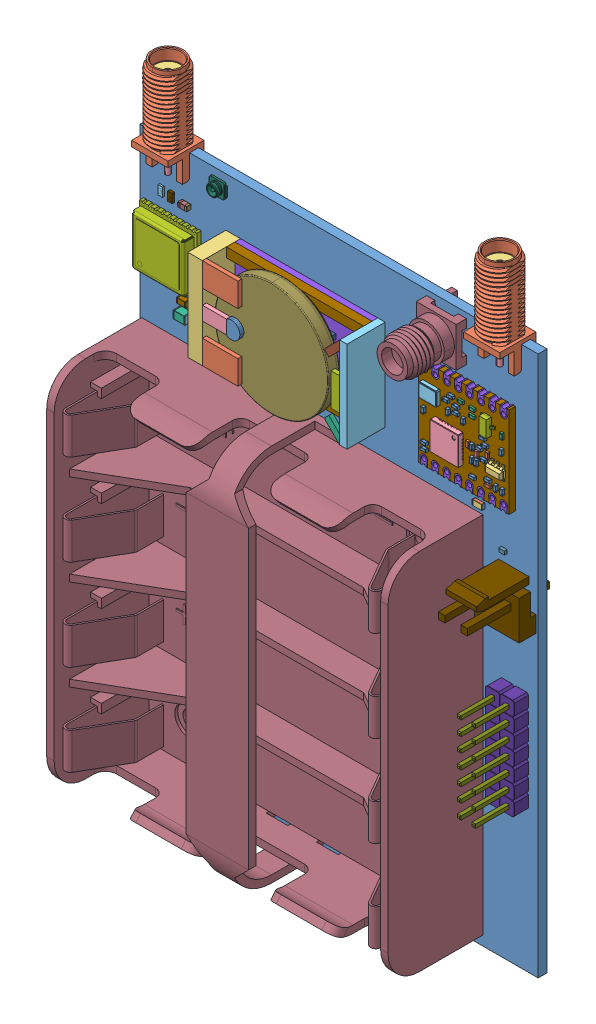
SolidWorks assembly Печатная плата Peggy Tracker степ, configuration По умолчанию. Lengths in mm.
Overall size (70 108.1 20.64).
358 component instances, 81 part files, 0 mates.
Components (placement in the parent):
- Печатная плата Peggy Tracker.step-1: Печатная плата Peggy Tracker.step [Default] at origin size (70 108.1 20.64)
  - Board.step-1: Board.step [Default] at origin size (70 95 1.56)
    - Open CASCADE STEP translator 6.8 1.1.1.step-1: Open CASCADE STEP translator 6.8 1.1.1.step [Default] at (0 0 -1.5596) size (70 95 1.56)
  - XW4.step-1: XW4.step [Default] at origin size (6.87 17.48 6.87)
    - SMA_female_edge_6.5x6.5.step-1: SMA_female_edge_6.5x6.5.step [Default] at (63.8984 92.1251 0.2) x (-1 0 0) z (0 0 1) size (6.87 17.48 6.87)
      - SMA_female_edge_6.5x6.5(2)^SMA_female_edge_6.5x6.5.step-1: SMA_female_edge_6.5x6.5(2)^SMA_female_edge_6.5x6.5.step [Default] at origin size (6.87 17.48 6.87)
        - Body^SMA_female_edge_6.5x6.5(2)_SMA_female_edge_6.5x6.5.step-1: Body^SMA_female_edge_6.5x6.5(2)_SMA_female_edge_6.5x6.5.step [Default] at (0 -4 0.45) x (0 0 1) z (0 -1 0) size (6.87 6.87 17.29)
        - Dielectric^SMA_female_edge_6.5x6.5(2)_SMA_female_edge_6.5x6.5.step-1: Dielectric^SMA_female_edge_6.5x6.5(2)_SMA_female_edge_6.5x6.5.step [Default] at (0 -4 0.45) x (0 0 1) z (0 -1 0) size (4.25 4.25 11.54)
        - Pin^SMA_female_edge_6.5x6.5(2)_SMA_female_edge_6.5x6.5.step-1: Pin^SMA_female_edge_6.5x6.5(2)_SMA_female_edge_6.5x6.5.step [Default] at (0 -4 0.45) x (0 0 1) z (0 -1 0) size (1.27 1.27 15.54)
  - C21.step-1: C21.step [Default] at origin size (1.6 0.8 0.3)
    - SW3dPS-0603_SMD_Capacitor.step-1: SW3dPS-0603_SMD_Capacitor.step [Default] at (25.6001 31.0999 -1.5596) x (1 0 0) z (0 1 0) size (1.6 0.3 0.8)
  - C20.step-1: C20.step [Default] at origin size (3.2 1.6 1)
    - SW3dPS-1206_SMD_Capacitor.step-1: SW3dPS-1206_SMD_Capacitor.step [Default] at (30.5 25 -1.5596) x (1 0 0) z (0 1 0) size (3.2 1 1.6)
  - C19.step-1: C19.step [Default] at origin size (1.6 0.8 0.3)
    - SW3dPS-0603_SMD_Capacitor.step-1: SW3dPS-0603_SMD_Capacitor.step [Default] at (27.9999 46.9001 -1.5596) x (-1 0 0) z (0 -1 0) size (1.6 0.3 0.8)
  - C18.step-1: C18.step [Default] at origin size (0.8 1.6 0.3)
    - SW3dPS-0603_SMD_Capacitor.step-1: SW3dPS-0603_SMD_Capacitor.step [Default] at (40.0999 43.0999 -1.5596) x (0 -1 0) z (1 0 0) size (1.6 0.3 0.8)
  - C17.step-1: C17.step [Default] at origin size (0.8 1.6 0.3)
    - SW3dPS-0603_SMD_Capacitor.step-1: SW3dPS-0603_SMD_Capacitor.step [Default] at (39.9001 34.9001 -1.5596) x (0 1 0) z (-1 0 0) size (1.6 0.3 0.8)
  - C16.step-1: C16.step [Default] at origin size (1.6 0.8 0.3)
    - SW3dPS-0603_SMD_Capacitor.step-1: SW3dPS-0603_SMD_Capacitor.step [Default] at (22.1999 32.8001 -1.5596) x (-1 0 0) z (0 -1 0) size (1.6 0.3 0.8)
  - DD1.step-1: DD1.step [Default] at origin size (10.1 9.7 2.7)
    - MAX-M8C-0.step-1: MAX-M8C-0.step [Default] at (5.7001 79.2999 0) x (0 1 0) z (1 0 0) size (9.7 2.7 10.1)
  - ZQ2.step-1: ZQ2.step [Default] at origin size (3.22 1.52 0.91)
    - User_Library-ABS07.step-1: User_Library-ABS07.step [Default] at (18.5999 54.9001 -1.5596) x (-1 0 0) z (0 -1 0) size (3.22 0.91 1.52)
      - User_Library-ABS07_ABS07_Body_2.step-1: User_Library-ABS07_ABS07_Body_2.step [Default] x (1 0 0) z (0 1 0) size (3.2 1.5 0.85)
      - User_Library-ABS07_ABS07_Body2_2.step-1: User_Library-ABS07_ABS07_Body2_2.step [Default] x (-1 0 0) z (0 1 0) size (3 1.3 0.05)
      - User_Library-ABS07_ABS07_Beschriftung_2.step-1: User_Library-ABS07_ABS07_Beschriftung_2.step [Default] x (-1 0 0) z (0 1 0) size (2.05 0.49 0.06)
      - User_Library-ABS07_ABS07_Pads_2.step-1: User_Library-ABS07_ABS07_Pads_2.step [Default] x (1 0 0) z (0 1 0) size (3.22 1.52 0.25)
  - ZQ1.step-1: ZQ1.step [Default] at origin size (3.18 5 1.11)
    - ABM3B.step-1: ABM3B.step [Default] at (21.4001 38.8001 -1.5596) x (0 -1 0) z (1 0 0) size (5 1.11 3.17)
  - XW3.step-1: XW3.step [Default] at origin size (7.01 7.53 13.48)
    - SMA_connector.step-1: SMA_connector.step [Default] at (53.9001 90.6 0) size (7.01 7.53 13.48)
      - User_Library-SMA_Stehend_Amp_132134RP-1_1.step-1: User_Library-SMA_Stehend_Amp_132134RP-1_1.step [Default] at origin size (7.01 7.53 13.48)
      - User_Library-SMA_Stehend_Amp_132134RP-1_2.step-1: User_Library-SMA_Stehend_Amp_132134RP-1_2.step [Default] at origin size (1.27 1.27 4.71)
  - XW2.step-1: XW2.step [Default] at origin size (3.01 2.86 1.29)
    - IPX.step-1: IPX.step [Default] at (13.8501 92.4001 1.27) size (3.01 2.86 1.29)
  - XW1.step-1: XW1.step [Default] at origin size (6.87 17.48 6.87)
    - SMA_female_edge_6.5x6.5.step-1: SMA_female_edge_6.5x6.5.step [Default] at (5.5484 92.1251 0.2) x (-1 0 0) z (0 0 1) size (6.87 17.48 6.87)
      - SMA_female_edge_6.5x6.5(2)^SMA_female_edge_6.5x6.5.step-1: SMA_female_edge_6.5x6.5(2)^SMA_female_edge_6.5x6.5.step [Default] at origin size (6.87 17.48 6.87)
        - Body^SMA_female_edge_6.5x6.5(2)_SMA_female_edge_6.5x6.5.step-1: Body^SMA_female_edge_6.5x6.5(2)_SMA_female_edge_6.5x6.5.step [Default] at (0 -4 0.45) x (0 0 1) z (0 -1 0) size (6.87 6.87 17.29)
        - Dielectric^SMA_female_edge_6.5x6.5(2)_SMA_female_edge_6.5x6.5.step-1: Dielectric^SMA_female_edge_6.5x6.5(2)_SMA_female_edge_6.5x6.5.step [Default] at (0 -4 0.45) x (0 0 1) z (0 -1 0) size (4.25 4.25 11.54)
        - Pin^SMA_female_edge_6.5x6.5(2)_SMA_female_edge_6.5x6.5.step-1: Pin^SMA_female_edge_6.5x6.5(2)_SMA_female_edge_6.5x6.5.step [Default] at (0 -4 0.45) x (0 0 1) z (0 -1 0) size (1.27 1.27 15.54)
  - X5.step-1: X5.step [Default] at origin size (5.08 17.78 11.54)
    - PLD-14.step-1: PLD-14.step [Default] at (64.5301 25.9799 0) x (0 -1 0) z (0 0 1) size (17.78 5.08 11.54)
      - ____________.step-1: ____________.step [Default] at (-12.7 0 -3) size (0.64 0.64 11.54)
      - _________.step-1: _________.step [Default] at (-5.1324 2.5342 -0.0112) size (2.54 2.54 2.54)
      - ____________.step-2: ____________.step [Default] at (-7.62 2.54 -3) size (0.64 0.64 11.54)
      - _________.step-2: _________.step [Default] at (-12.7524 -0.0058 -0.0112) size (2.54 2.54 2.54)
      - ____________.step-3: ____________.step [Default] at (-15.24 2.54 -3) size (0.64 0.64 11.54)
      - _________.step-3: _________.step [Default] at (-10.2124 2.5342 -0.0112) size (2.54 2.54 2.54)
      - ____________.step-4: ____________.step [Default] at (-12.7 2.54 -3) size (0.64 0.64 11.54)
      - ____________.step-5: ____________.step [Default] at (-10.16 2.54 -3) size (0.64 0.64 11.54)
      - ____________.step-6: ____________.step [Default] at (-15.24 0 -3) size (0.64 0.64 11.54)
      - ____________.step-7: ____________.step [Default] at (0 2.54 -3) size (0.64 0.64 11.54)
      - ____________.step-8: ____________.step [Default] at (-7.62 0 -3) size (0.64 0.64 11.54)
      - _________.step-4: _________.step [Default] at (-5.1324 -0.0058 -0.0112) size (2.54 2.54 2.54)
      - _________.step-5: _________.step [Default] at (-2.5924 -0.0058 -0.0112) size (2.54 2.54 2.54)
      - ____________.step-9: ____________.step [Default] at (-2.54 0 -3) size (0.64 0.64 11.54)
      - ____________.step-10: ____________.step [Default] at (-5.08 0 -3) size (0.64 0.64 11.54)
      - _________.step-6: _________.step [Default] at (-0.0524 2.5342 -0.0112) size (2.54 2.54 2.54)
      - _________.step-7: _________.step [Default] at (-7.6724 2.5342 -0.0112) size (2.54 2.54 2.54)
      - ____________.step-11: ____________.step [Default] at (-5.08 2.54 -3) size (0.64 0.64 11.54)
      - _________.step-8: _________.step [Default] at (-7.6724 -0.0058 -0.0112) size (2.54 2.54 2.54)
      - _________.step-9: _________.step [Default] at (-15.2924 2.5342 -0.0112) size (2.54 2.54 2.54)
      - ____________.step-12: ____________.step [Default] at (-2.54 2.54 -3) size (0.64 0.64 11.54)
      - ____________.step-13: ____________.step [Default] at (0 0 -3) size (0.64 0.64 11.54)
      - _________.step-10: _________.step [Default] at (-10.2124 -0.0058 -0.0112) size (2.54 2.54 2.54)
      - _________.step-11: _________.step [Default] at (-15.2924 -0.0058 -0.0112) size (2.54 2.54 2.54)
      - _________.step-12: _________.step [Default] at (-2.5924 2.5342 -0.0112) size (2.54 2.54 2.54)
      - _________.step-13: _________.step [Default] at (-12.7524 2.5342 -0.0112) size (2.54 2.54 2.54)
      - _________.step-14: _________.step [Default] at (-0.0524 -0.0058 -0.0112) size (2.54 2.54 2.54)
      - ____________.step-14: ____________.step [Default] at (-10.16 0 -3) size (0.64 0.64 11.54)
  - X4.step-1: X4.step [Default] at origin size (7.86 8.5 14.4)
    - 1-1123723-2.step-1: 1-1123723-2.step [Default] at (65.7 57.0999 3) x (1 0 0) z (0 0 1) size (7.86 8.5 14.4)
  - X2.step-1: X2.step [Default] at origin size (28 20 6.7)
    - 6036059248.step-1: 6036059248.step [Default] at (22.75 78.4 6) size (3 3 0.7)
      - Extruded.step-1: Extruded.step [Default] at origin size (3 3 0.7)
    - 6036054288.step-1: 6036054288.step [Default] at (20.7815 72.4945 6) size (6.22 4.19 0.7)
      - Extruded-0.step-1: Extruded-0.step [Default] at origin size (6.22 4.19 0.7)
    - 6036054288.step-2: 6036054288.step [Default] at (20.7815 84.3045 6) size (6.22 4.19 0.7)
      - Extruded-0.step-1: Extruded-0.step [Default] at origin size (6.22 4.19 0.7)
    - 6036054608.step-1: 6036054608.step [Default] at (16.385 78.3995 0) size (2.57 16 6.7)
      - Extruded-1.step-1: Extruded-1.step [Default] at origin size (2.57 16 6.7)
    - 6036055008.step-1: 6036055008.step [Default] at (19.7818 78.4135 6) size (4.22 2.41 0.7)
      - Extruded-2.step-1: Extruded-2.step [Default] at origin size (4.22 2.41 0.7)
    - 6036055248.step-1: 6036055248.step [Default] at (42.4492 78.3995 0) size (1.3 16 6.7)
      - Extruded-3.step-1: Extruded-3.step [Default] at origin size (1.3 16 6.7)
    - 6036055568.step-1: 6036055568.step [Default] at (40.5305 72.1757 6) size (2.54 3.55 0.7)
      - Extruded-4.step-1: Extruded-4.step [Default] at origin size (2.54 3.55 0.7)
    - 6036055968.step-1: 6036055968.step [Default] at (41.0382 78.0825 6) size (1.52 5.71 0.7)
      - Extruded-5.step-1: Extruded-5.step [Default] at origin size (1.52 5.71 0.7)
    - 6036056288.step-1: 6036056288.step [Default] at (29.7354 78.3995 0) size (24.13 16 1)
      - Extruded-6.step-1: Extruded-6.step [Default] at origin size (24.13 16 1)
    - 6036056848.step-1: 6036056848.step [Default] at (29.735 85.575 0) size (24.13 1.65 2.5)
      - Extruded-7.step-1: Extruded-7.step [Default] at origin size (24.13 1.65 2.5)
    - 6036056848.step-2: 6036056848.step [Default] at (29.7356 71.2237 0) size (24.13 1.65 2.5)
      - Extruded-7.step-1: Extruded-7.step [Default] at origin size (24.13 1.65 2.5)
    - 6036057568.step-1: 6036057568.step [Default] at (30.6875 75.4163 0) size (9.53 0.89 2.5)
      - Extruded-8.step-1: Extruded-8.step [Default] at origin size (9.53 0.89 2.5)
    - 6036057568.step-2: 6036057568.step [Default] at (30.6875 80.8773 0) size (9.53 0.89 2.5)
      - Extruded-8.step-1: Extruded-8.step [Default] at origin size (9.53 0.89 2.5)
    - 6036057888.step-1: 6036057888.step [Default] at (40.5302 84.622 6) size (2.54 3.55 0.7)
      - Extruded-9.step-1: Extruded-9.step [Default] at origin size (2.54 3.55 0.7)
    - CircuitWorks-BATT_CR2032.step-1: CircuitWorks-BATT_CR2032.step [Default] at (29.1 78.4 6) x (1 0 0) z (0 1 0) size (20 3.2 20)
  - X1.step-1: X1.step [Default] at origin size (60 66.54 19.72)
    - BK-1279-PC8--3DModel-STEP-56544.step-1: BK-1279-PC8--3DModel-STEP-56544.step [Default] at (30.3 33.7 -3.02) x (-1 0 0) z (0 1 0) size (60 19.72 66.54)
  - VD1.step-1: VD1.step [Default] at origin size (1 0.6 0.53)
    - DESD3V3S1BL-7B.step-1: DESD3V3S1BL-7B.step [Default] at (64.05 62.2 0) x (1 0 0) z (0 -1 0) size (1 0.53 0.6)
  - R9.step-1: R9.step [Default] at origin size (0.9 1.7 0.55)
    - 5945467952.step-1: 5945467952.step [Default] at (35.1001 47.7001 -1.5596) x (0 1 0) z (0 0 -1) size (1.7 0.9 0.55)
      - Terminal.step-1: Terminal.step [Default] at (-0.85 -0.45 0) size (0.1 0.9 0.55)
        - Open_CASCADE_STEP_translator_6.8_15.2.1.step-1: Open_CASCADE_STEP_translator_6.8_15.2.1.step [Default] at origin size (0.1 0.9 0.55)
      - Terminal.step-2: Terminal.step [Default] at (0.85 0.45 0) x (-1 0 0) z (0 0 1) size (0.1 0.9 0.55)
        - Open_CASCADE_STEP_translator_6.8_15.2.1.step-1: Open_CASCADE_STEP_translator_6.8_15.2.1.step [Default] at origin size (0.1 0.9 0.55)
      - Mid_Body.step-1: Mid_Body.step [Default] at (-0.85 -0.45 0) size (1.59 0.9 0.44)
      - Mark.step-1: Mark.step [Default] at (-0.75 -0.45 0.495) size (1.5 0.9 0.06)
  - R8.step-1: R8.step [Default] at origin size (0.81 1.61 0.46)
    - chip_0603_r.step-1: chip_0603_r.step [Default] at (41.6999 34.1001 -1.7696) x (-1 0 0) z (0 0 -1) size (0.81 1.61 0.46)
  - R7.step-1: R7.step [Default] at origin size (1.7 0.9 0.55)
    - 5945464112.step-1: 5945464112.step [Default] at (59.8001 67.2001 0) size (1.7 0.9 0.55)
      - Terminal-1.step-1: Terminal-1.step [Default] at (-0.85 -0.45 0) size (0.1 0.9 0.55)
        - Open_CASCADE_STEP_translator_6.8_15.2.1-10.step-1: Open_CASCADE_STEP_translator_6.8_15.2.1-10.step [Default] at origin size (0.1 0.9 0.55)
      - Terminal-1.step-2: Terminal-1.step [Default] at (0.85 0.45 0) x (-1 0 0) z (0 0 1) size (0.1 0.9 0.55)
        - Open_CASCADE_STEP_translator_6.8_15.2.1-10.step-1: Open_CASCADE_STEP_translator_6.8_15.2.1-10.step [Default] at origin size (0.1 0.9 0.55)
      - Mid_Body-11.step-1: Mid_Body-11.step [Default] at (-0.85 -0.45 0) size (1.59 0.9 0.44)
      - Mark-12.step-1: Mark-12.step [Default] at (-0.75 -0.45 0.495) size (1.5 0.9 0.06)
  - R6.step-1: R6.step [Default] at origin size (1.61 0.81 0.46)
    - chip_0603_r.step-1: chip_0603_r.step [Default] at (40.2001 37.4001 -1.7696) x (0 1 0) z (0 0 -1) size (0.81 1.61 0.46)
  - R5.step-1: R5.step [Default] at origin size (1.61 0.81 0.46)
    - chip_0603_r.step-1: chip_0603_r.step [Default] at (24.8999 29.2999 -1.7696) x (0 -1 0) z (0 0 -1) size (0.81 1.61 0.46)
  - R4.step-1: R4.step [Default] at origin size (1.61 0.81 0.46)
    - chip_0603_r.step-1: chip_0603_r.step [Default] at (18.0999 22.9999 -1.7696) x (0 -1 0) z (0 0 -1) size (0.81 1.61 0.46)
  - R3.step-1: R3.step [Default] at origin size (0.81 1.61 0.46)
    - chip_0603_r.step-1: chip_0603_r.step [Default] at (20.5999 17.2001 -1.7696) x (-1 0 0) z (0 0 -1) size (0.81 1.61 0.46)
  - R2.step-1: R2.step [Default] at origin size (1.61 0.81 0.46)
    - chip_0603_r.step-1: chip_0603_r.step [Default] at (14.1999 22.9999 -1.7696) x (0 -1 0) z (0 0 -1) size (0.81 1.61 0.46)
  - R1.step-1: R1.step [Default] at origin size (0.81 1.61 0.46)
    - chip_0603_r.step-1: chip_0603_r.step [Default] at (5.675 87.7 0.21) x (-1 0 0) z (0 0 1) size (0.81 1.61 0.46)
  - MPU1.step-1: MPU1.step [Default] at origin size (12 12 1.2)
    - 5945464032.step-1: 5945464032.step [Default] at (31.9001 39.0001 -1.5596) x (0 1 0) z (0 0 -1) size (12 12 1.2)
      - Body.step-1: Body.step [Default] at (-5 -5 0) size (10.01 10.01 1.15)
        - Open_CASCADE_STEP_translator_6.8_62.2.1.step-1: Open_CASCADE_STEP_translator_6.8_62.2.1.step [Default] at origin size (10.01 10.01 1.15)
      - Open_CASCADE_STEP_translator_6.8_62.1.step-1: Open_CASCADE_STEP_translator_6.8_62.1.step [Default] at (-5 -5 0.001) size (1.26 1.26 0.01)
      - Leader.step-1: Leader.step [Default] at (-5 -4 0) x (-1 0 0) z (0 0 1) size (1 0.38 0.68)
      - Leader.step-2: Leader.step [Default] at (-5 -3.2 0) x (-1 0 0) z (0 0 1) size (1 0.38 0.68)
      - Leader.step-3: Leader.step [Default] at (-5 -2.4 0) x (-1 0 0) z (0 0 1) size (1 0.38 0.68)
      - Leader.step-4: Leader.step [Default] at (-5 -1.6 0) x (-1 0 0) z (0 0 1) size (1 0.38 0.68)
      - Leader.step-5: Leader.step [Default] at (-5 -0.8 0) x (-1 0 0) z (0 0 1) size (1 0.38 0.68)
      - Leader.step-6: Leader.step [Default] at (-5 0 0) x (-1 0 0) z (0 0 1) size (1 0.38 0.68)
      - Leader.step-7: Leader.step [Default] at (-5 0.8 0) x (-1 0 0) z (0 0 1) size (1 0.38 0.68)
      - Leader.step-8: Leader.step [Default] at (-5 1.6 0) x (-1 0 0) z (0 0 1) size (1 0.38 0.68)
      - Leader.step-9: Leader.step [Default] at (-5 2.4 0) x (-1 0 0) z (0 0 1) size (1 0.38 0.68)
      - Leader.step-10: Leader.step [Default] at (-5 3.2 0) x (-1 0 0) z (0 0 1) size (1 0.38 0.68)
      - Leader.step-11: Leader.step [Default] at (-5 4 0) x (-1 0 0) z (0 0 1) size (1 0.38 0.68)
      - Leader.step-12: Leader.step [Default] at (5 -4 0) size (1 0.38 0.68)
      - Leader.step-13: Leader.step [Default] at (5 -3.2 0) size (1 0.38 0.68)
      - Leader.step-14: Leader.step [Default] at (5 -2.4 0) size (1 0.38 0.68)
      - Leader.step-15: Leader.step [Default] at (5 -1.6 0) size (1 0.38 0.68)
      - Leader.step-16: Leader.step [Default] at (5 -0.8 0) size (1 0.38 0.68)
      - Leader.step-17: Leader.step [Default] at (5 0 0) size (1 0.38 0.68)
      - Leader.step-18: Leader.step [Default] at (5 0.8 0) size (1 0.38 0.68)
      - Leader.step-19: Leader.step [Default] at (5 1.6 0) size (1 0.38 0.68)
      - Leader.step-20: Leader.step [Default] at (5 2.4 0) size (1 0.38 0.68)
      - Leader.step-21: Leader.step [Default] at (5 3.2 0) size (1 0.38 0.68)
      - Leader.step-22: Leader.step [Default] at (5 4 0) size (1 0.38 0.68)
      - Leader-13.step-1: Leader-13.step [Default] at (-4 -5 0) x (0 -1 0) z (0 0 1) size (1 0.38 0.68)
      - Leader-13.step-2: Leader-13.step [Default] at (-3.2 -5 0) x (0 -1 0) z (0 0 1) size (1 0.38 0.68)
      - Leader-13.step-3: Leader-13.step [Default] at (-2.4 -5 0) x (0 -1 0) z (0 0 1) size (1 0.38 0.68)
      - Leader-13.step-4: Leader-13.step [Default] at (-1.6 -5 0) x (0 -1 0) z (0 0 1) size (1 0.38 0.68)
      - Leader-13.step-5: Leader-13.step [Default] at (-0.8 -5 0) x (0 -1 0) z (0 0 1) size (1 0.38 0.68)
      - Leader-13.step-6: Leader-13.step [Default] at (0 -5 0) x (0 -1 0) z (0 0 1) size (1 0.38 0.68)
      - Leader-13.step-7: Leader-13.step [Default] at (0.8 -5 0) x (0 -1 0) z (0 0 1) size (1 0.38 0.68)
      - Leader-13.step-8: Leader-13.step [Default] at (1.6 -5 0) x (0 -1 0) z (0 0 1) size (1 0.38 0.68)
      - Leader-13.step-9: Leader-13.step [Default] at (2.4 -5 0) x (0 -1 0) z (0 0 1) size (1 0.38 0.68)
      - Leader-13.step-10: Leader-13.step [Default] at (3.2 -5 0) x (0 -1 0) z (0 0 1) size (1 0.38 0.68)
      - Leader-13.step-11: Leader-13.step [Default] at (4 -5 0) x (0 -1 0) z (0 0 1) size (1 0.38 0.68)
      - Leader-13.step-12: Leader-13.step [Default] at (-4 5 0) x (0 1 0) z (0 0 1) size (1 0.38 0.68)
      - Leader-13.step-13: Leader-13.step [Default] at (-3.2 5 0) x (0 1 0) z (0 0 1) size (1 0.38 0.68)
      - Leader-13.step-14: Leader-13.step [Default] at (-2.4 5 0) x (0 1 0) z (0 0 1) size (1 0.38 0.68)
      - Leader-13.step-15: Leader-13.step [Default] at (-1.6 5 0) x (0 1 0) z (0 0 1) size (1 0.38 0.68)
      - Leader-13.step-16: Leader-13.step [Default] at (-0.8 5 0) x (0 1 0) z (0 0 1) size (1 0.38 0.68)
      - Leader-13.step-17: Leader-13.step [Default] at (0 5 0) x (0 1 0) z (0 0 1) size (1 0.38 0.68)
      - Leader-13.step-18: Leader-13.step [Default] at (0.8 5 0) x (0 1 0) z (0 0 1) size (1 0.38 0.68)
      - Leader-13.step-19: Leader-13.step [Default] at (1.6 5 0) x (0 1 0) z (0 0 1) size (1 0.38 0.68)
      - Leader-13.step-20: Leader-13.step [Default] at (2.4 5 0) x (0 1 0) z (0 0 1) size (1 0.38 0.68)
      - Leader-13.step-21: Leader-13.step [Default] at (3.2 5 0) x (0 1 0) z (0 0 1) size (1 0.38 0.68)
      - Leader-13.step-22: Leader-13.step [Default] at (4 5 0) x (0 1 0) z (0 0 1) size (1 0.38 0.68)
    - User_Library-VQFN(44).step-1: User_Library-VQFN(44).step [Default] at (28.3541 42.5231 -1.5596) x (1 0 0) z (0 1 0) size (7.1 0.95 7.1)
  - L3.step-1: L3.step [Default] at origin size (1.25 2 0.85)
    - User_Library-FB_2012-1.step-1: User_Library-FB_2012-1.step [Default] at (29.1001 21.7001 -1.5596) x (0 1 0) z (0 0 -1) size (2 1.25 0.85)
      - User_Library-FB_2012-1_Pad001.step-1: User_Library-FB_2012-1_Pad001.step [Default] at (0 0 0.03) size (1.94 1.19 0.79)
      - User_Library-FB_2012-1_Cut.step-1: User_Library-FB_2012-1_Cut.step [Default] at origin size (2 1.25 0.85)
  - L2.step-1: L2.step [Default] at origin size (2 1.25 0.85)
    - User_Library-FB_2012-1.step-1: User_Library-FB_2012-1.step [Default] at (56.1999 81.8001 -1.5596) x (-1 0 0) z (0 0 -1) size (2 1.25 0.85)
      - User_Library-FB_2012-1_Pad001.step-1: User_Library-FB_2012-1_Pad001.step [Default] at (0 0 0.03) size (1.94 1.19 0.79)
      - User_Library-FB_2012-1_Cut.step-1: User_Library-FB_2012-1_Cut.step [Default] at origin size (2 1.25 0.85)
  - L1.step-1: L1.step [Default] at origin size (1.6 0.8 0.8)
    - 5945464832.step-1: 5945464832.step [Default] at (8.2 86.9 0) size (1.6 0.8 0.8)
      - Terminal-2.step-1: Terminal-2.step [Default] at (-0.8 -0.4 0) size (1.6 0.8 0.8)
        - Open_CASCADE_STEP_translator_6.8_17.1.1.step-1: Open_CASCADE_STEP_translator_6.8_17.1.1.step [Default] at origin size (0.4 0.8 0.8)
        - Open_CASCADE_STEP_translator_6.8_17.1.2.step-1: Open_CASCADE_STEP_translator_6.8_17.1.2.step [Default] at origin size (0.4 0.8 0.8)
      - Mid_Body-14.step-1: Mid_Body-14.step [Default] at (-0.8 -0.4 0) size (0.8 0.8 0.8)
        - Open_CASCADE_STEP_translator_6.8_17.2.1.step-1: Open_CASCADE_STEP_translator_6.8_17.2.1.step [Default] at origin size (0.8 0.8 0.8)
  - HL1.step-1: HL1.step [Default] at origin size (0.81 1.61 0.61)
    - User_Library-LED_0603_G.step-1: User_Library-LED_0603_G.step [Default] at (37.1999 47.7999 -1.5596) x (0 -1 0) z (0 0 -1) size (1.61 0.81 0.61)
      - User_Library-LED_0603_G_Pocket002.step-1: User_Library-LED_0603_G_Pocket002.step [Default] at origin size (0.41 0.81 0.21)
      - User_Library-LED_0603_G_Pad004.step-1: User_Library-LED_0603_G_Pad004.step [Default] x (1 0 0) z (0 0 -1) size (0.4 0.8 0)
      - User_Library-LED_0603_G_Fillet.step-1: User_Library-LED_0603_G_Fillet.step [Default] at origin size (1 0.7 0.4)
      - User_Library-LED_0603_G_Pocket001.step-1: User_Library-LED_0603_G_Pocket001.step [Default] at origin size (0.4 0.8 0.2)
      - User_Library-LED_0603_G_Pad.step-1: User_Library-LED_0603_G_Pad.step [Default] at origin size (0.8 0.8 0.2)
  - DD2.step-1: DD2.step [Default] at origin size (15.9 16 2.23)
    - User_Library-RFM96W.step-1: User_Library-RFM96W.step [Default] at (50.075 85.102 1.15) x (0 -1 0) z (0 0 1) size (16 15.9 2.23)
      - Designator4.step-1: Designator4.step [Default] at origin size (0.5 1 0.5)
        - Cap0402.step-1: Cap0402.step [Default] at (13.208 1.27 0) x (0 -1 0) z (-1 0 0) size (1 0.5 0.5)
      - Designator6.step-1: Designator6.step [Default] at origin size (1 0.5 0.5)
        - Cap0402.step-1: Cap0402.step [Default] at (7.239 1.143 0) x (-1 0 0) z (0 1 0) size (1 0.5 0.5)
      - Designator7.step-1: Designator7.step [Default] at origin size (0.5 1 0.5)
        - Cap0402.step-1: Cap0402.step [Default] at (3.81 5.08 0) x (0 -1 0) z (-1 0 0) size (1 0.5 0.5)
      - Designator8.step-1: Designator8.step [Default] at origin size (1 0.5 0.5)
        - Cap0402.step-1: Cap0402.step [Default] at (5.4 5.45 0) x (1 0 0) z (0 -1 0) size (1 0.5 0.5)
      - Designator9.step-1: Designator9.step [Default] at origin size (0.5 1 0.5)
        - Cap0402.step-1: Cap0402.step [Default] at (2.8 5.98 0) x (0 -1 0) z (-1 0 0) size (1 0.5 0.5)
      - Designator10.step-1: Designator10.step [Default] at origin size (0.5 1 0.5)
        - Cap0402.step-1: Cap0402.step [Default] at (4.953 6.858 0) x (0 -1 0) z (-1 0 0) size (1 0.5 0.5)
      - Designator11.step-1: Designator11.step [Default] at origin size (0.5 1 0.5)
        - Cap0402.step-1: Cap0402.step [Default] at (6.35 11.557 0) x (0 1 0) z (1 0 0) size (1 0.5 0.5)
      - Designator12.step-1: Designator12.step [Default] at origin size (1 0.5 0.5)
        - Cap0402.step-1: Cap0402.step [Default] at (5.461 8.128 0) x (1 0 0) z (0 -1 0) size (1 0.5 0.5)
      - Designator13.step-1: Designator13.step [Default] at origin size (0.5 1 0.5)
        - Cap0402.step-1: Cap0402.step [Default] at (3.937 6.858 0) x (0 1 0) z (1 0 0) size (1 0.5 0.5)
      - Designator15.step-1: Designator15.step [Default] at origin size (0.52 1.02 0.37)
        - SW3dPS-inductor_0402_white.step-1: SW3dPS-inductor_0402_white.step [Default] at (13.208 12.446 0) x (1 0 0) z (0 -1 0) size (0.52 0.37 1.02)
      - Designator17.step-1: Designator17.step [Default] at origin size (1.02 0.52 0.37)
        - SW3dPS-inductor_0402_white.step-1: SW3dPS-inductor_0402_white.step [Default] at (8.636 8.89 0) x (0 1 0) z (1 0 0) size (0.52 0.37 1.02)
      - Designator18.step-1: Designator18.step [Default] at origin size (1.02 0.52 0.37)
        - SW3dPS-inductor_0402_white.step-1: SW3dPS-inductor_0402_white.step [Default] at (9.398 10.414 0) x (0 1 0) z (1 0 0) size (0.52 0.37 1.02)
      - Designator19.step-1: Designator19.step [Default] at origin size (1.02 0.52 0.37)
        - SW3dPS-inductor_0402_white.step-1: SW3dPS-inductor_0402_white.step [Default] at (8.636 12.319 0) x (0 1 0) z (1 0 0) size (0.52 0.37 1.02)
      - Designator20.step-1: Designator20.step [Default] at origin size (1.02 0.52 0.37)
        - SW3dPS-inductor_0402_white.step-1: SW3dPS-inductor_0402_white.step [Default] at (10.668 12.319 0) x (0 1 0) z (1 0 0) size (0.52 0.37 1.02)
      - Designator21.step-1: Designator21.step [Default] at origin size (1 0.5 0.5)
        - Cap0402.step-1: Cap0402.step [Default] at (10.668 10.414 0) x (-1 0 0) z (0 1 0) size (1 0.5 0.5)
      - Designator22.step-1: Designator22.step [Default] at origin size (0.5 1 0.5)
        - Cap0402.step-1: Cap0402.step [Default] at (8.255 10.922 0) x (0 1 0) z (1 0 0) size (1 0.5 0.5)
      - Designator23.step-1: Designator23.step [Default] at origin size (1 0.5 0.5)
        - Cap0402.step-1: Cap0402.step [Default] at (6.858 14.859 0) x (-1 0 0) z (0 1 0) size (1 0.5 0.5)
      - Designator24.step-1: Designator24.step [Default] at origin size (1 0.5 0.5)
        - Cap0402.step-1: Cap0402.step [Default] at (12.827 13.843 0) x (-1 0 0) z (0 1 0) size (1 0.5 0.5)
      - Designator25.step-1: Designator25.step [Default] at origin size (0.5 1 0.5)
        - Cap0402.step-1: Cap0402.step [Default] at (7.366 11.938 0) x (0 -1 0) z (-1 0 0) size (1 0.5 0.5)
      - Designator26.step-1: Designator26.step [Default] at origin size (0.5 1 0.5)
        - Cap0402.step-1: Cap0402.step [Default] at (12.319 12.446 0) x (0 -1 0) z (-1 0 0) size (1 0.5 0.5)
      - Designator27.step-1: Designator27.step [Default] at origin size (1 0.5 0.5)
        - Cap0402.step-1: Cap0402.step [Default] at (12.827 14.986 0) x (-1 0 0) z (0 1 0) size (1 0.5 0.5)
      - Designator28.step-1: Designator28.step [Default] at origin size (0.5 1 0.5)
        - Cap0402.step-1: Cap0402.step [Default] at (9.652 11.684 0) x (0 -1 0) z (-1 0 0) size (1 0.5 0.5)
      - Designator29.step-1: Designator29.step [Default] at origin size (0.5 1 0.5)
        - Cap0402.step-1: Cap0402.step [Default] at (13.208 9.779 0) x (0 -1 0) z (-1 0 0) size (1 0.5 0.5)
      - Designator27_2.step-1: Designator27_2.step [Default] at origin size (2.43 2.79 1.09)
        - SW3dPS-SOT-23-6.step-1: SW3dPS-SOT-23-6.step [Default] at (9.0742 15.0495 0) x (0 -1 0) z (0 0 1) size (2.79 2.43 1.09)
      - Designator2.step-1: Designator2.step [Default] at origin size (5.04 5.04 0.9)
        - QFN28.step-1: QFN28.step [Default] at (9.97 5.42 0) x (0 -1 0) z (-1 0 0) size (5.04 0.9 5.04)
      - Designator5.step-1: Designator5.step [Default] at origin size (0.5 1 0.5)
        - Cap0402.step-1: Cap0402.step [Default] at (12.192 1.27 0) x (0 -1 0) z (-1 0 0) size (1 0.5 0.5)
      - Designator1.step-1: Designator1.step [Default] at origin size (2.5 3.2 0.7)
        - TXC_7M.step-1: TXC_7M.step [Default] at (4.1911 2.286 0) x (0 1 0) z (1 0 0) size (3.2 0.7 2.5)
      - Open_CASCADE_STEP_translator_6.5_1.29.step-1: Open_CASCADE_STEP_translator_6.5_1.29.step [Default] at origin size (0.5 1 0.35)
        - Res0402.step-1: Res0402.step [Default] at (2.794 7.62 0) x (0 1 0) z (1 0 0) size (1 0.35 0.5)
      - 1.step-1: 1.step [Default] at origin size (0.5 1 0.35)
        - Res0402.step-1: Res0402.step [Default] at (2.921 9.652 0) x (0 1 0) z (1 0 0) size (1 0.35 0.5)
      - 2.step-1: 2.step [Default] at origin size (0.5 1 0.35)
        - Res0402.step-1: Res0402.step [Default] at (4.064 9.652 0) x (0 1 0) z (1 0 0) size (1 0.35 0.5)
      - Open_CASCADE_STEP_translator_6.5_1.32.step-1: Open_CASCADE_STEP_translator_6.5_1.32.step [Default] at origin size (3.03 2.48 1.12)
        - User_Library-3-lead_sot23-3.step-1: User_Library-3-lead_sot23-3.step [Default] at (3.9981 12.3031 0.35) x (1 0 0) z (0 -1 0) size (3.03 1.12 2.48)
      - 3.step-1: 3.step [Default] at origin size (1 0.5 0.35)
        - Res0402.step-1: Res0402.step [Default] at (4.445 14.859 0) x (-1 0 0) z (0 1 0) size (1 0.35 0.5)
      - Designator31.step-1: Designator31.step [Default] at origin size (1 0.5 0.5)
        - Cap0402.step-1: Cap0402.step [Default] at (8.636 9.652 0) x (-1 0 0) z (0 1 0) size (1 0.5 0.5)
      - Designator32.step-1: Designator32.step [Default] at origin size (1 0.5 0.5)
        - Cap0402.step-1: Cap0402.step [Default] at (10.668 9.652 0) x (-1 0 0) z (0 1 0) size (1 0.5 0.5)
      - Free-Models.step-1: Free-Models.step [Default] at origin size (16 15.3 1.16)
        - Goldcontact.step-1: Goldcontact.step [Default] at (0.56 1 -1.14) x (-1 0 0) z (0 1 0) size (1.77 1.16 1.3)
        - Goldcontact.step-2: Goldcontact.step [Default] at (0.56 3 -1.14) x (-1 0 0) z (0 1 0) size (1.77 1.16 1.3)
        - Goldcontact.step-3: Goldcontact.step [Default] at (0.56 5 -1.14) x (-1 0 0) z (0 1 0) size (1.77 1.16 1.3)
        - Goldcontact.step-4: Goldcontact.step [Default] at (0.56 7 -1.14) x (-1 0 0) z (0 1 0) size (1.77 1.16 1.3)
        - Goldcontact.step-5: Goldcontact.step [Default] at (0.56 9 -1.14) x (-1 0 0) z (0 1 0) size (1.77 1.16 1.3)
        - Goldcontact.step-6: Goldcontact.step [Default] at (0.56 11 -1.14) x (-1 0 0) z (0 1 0) size (1.77 1.16 1.3)
        - Goldcontact.step-7: Goldcontact.step [Default] at (0.56 13 -1.14) x (-1 0 0) z (0 1 0) size (1.77 1.16 1.3)
        - Goldcontact.step-8: Goldcontact.step [Default] at (0.56 15 -1.14) x (-1 0 0) z (0 1 0) size (1.77 1.16 1.3)
        - Goldcontact.step-9: Goldcontact.step [Default] at (15.442 15 -1.14) x (1 0 0) z (0 -1 0) size (1.77 1.16 1.3)
        - Goldcontact.step-10: Goldcontact.step [Default] at (15.442 13 -1.14) x (1 0 0) z (0 -1 0) size (1.77 1.16 1.3)
        - Goldcontact.step-11: Goldcontact.step [Default] at (15.442 11 -1.14) x (1 0 0) z (0 -1 0) size (1.77 1.16 1.3)
        - Goldcontact.step-12: Goldcontact.step [Default] at (15.442 9 -1.14) x (1 0 0) z (0 -1 0) size (1.77 1.16 1.3)
        - Goldcontact.step-13: Goldcontact.step [Default] at (15.442 7 -1.14) x (1 0 0) z (0 -1 0) size (1.77 1.16 1.3)
        - Goldcontact.step-14: Goldcontact.step [Default] at (15.442 5 -1.14) x (1 0 0) z (0 -1 0) size (1.77 1.16 1.3)
        - Goldcontact.step-15: Goldcontact.step [Default] at (15.442 3 -1.14) x (1 0 0) z (0 -1 0) size (1.77 1.16 1.3)
        - Goldcontact.step-16: Goldcontact.step [Default] at (15.442 1 -1.14) x (1 0 0) z (0 -1 0) size (1.77 1.16 1.3)
      - Board-15.step-1: Board-15.step [Default] at (0 0 -1.1204) size (15.9 15.9 1.12)
  - D2.step-1: D2.step [Default] at origin size (4.9 6 1.75)
    - User_Library-SOIC-8-1.step-1: User_Library-SOIC-8-1.step [Default] at (19.8999 49.3999 -1.5596) x (1 0 0) z (0 0 -1) size (4.9 6 1.75)
  - D1.step-1: D1.step [Default] at origin size (6.6 6.6 1.2)
    - TSSOP-20.step-1: TSSOP-20.step [Default] at (14.6001 18.2999 -1.5596) x (0 1 0) z (-1 0 0) size (6.6 1.2 6.6)
  - C15.step-1: C15.step [Default] at origin size (1.6 3.2 1)
    - SW3dPS-1206_SMD_Capacitor.step-1: SW3dPS-1206_SMD_Capacitor.step [Default] at (29.1 17.2 -1.5596) x (0 -1 0) z (1 0 0) size (3.2 1 1.6)
  - C14.step-1: C14.step [Default] at origin size (3.2 1.6 1)
    - SW3dPS-1206_SMD_Capacitor.step-1: SW3dPS-1206_SMD_Capacitor.step [Default] at (58.6 84.5 -1.5596) x (1 0 0) z (0 1 0) size (3.2 1 1.6)
  - C13.step-1: C13.step [Default] at origin size (0.8 1.6 0.3)
    - SW3dPS-0603_SMD_Capacitor.step-1: SW3dPS-0603_SMD_Capacitor.step [Default] at (15.5001 55.6001 -1.5596) x (0 1 0) z (-1 0 0) size (1.6 0.3 0.8)
  - C12.step-1: C12.step [Default] at origin size (0.8 1.6 0.3)
    - SW3dPS-0603_SMD_Capacitor.step-1: SW3dPS-0603_SMD_Capacitor.step [Default] at (21.6999 54.9999 -1.5596) x (0 -1 0) z (1 0 0) size (1.6 0.3 0.8)
  - C11.step-1: C11.step [Default] at origin size (1.7 0.9 0.9)
    - 5945466272.step-1: 5945466272.step [Default] at (17.1 44.6 -1.5596) x (1 0 0) z (0 0 -1) size (1.7 0.9 0.9)
      - Terminal-3.step-1: Terminal-3.step [Default] at (-0.85 -0.45 0) size (1.7 0.9 0.9)
        - Open_CASCADE_STEP_translator_6.8_5.1.1.step-1: Open_CASCADE_STEP_translator_6.8_5.1.1.step [Default] at origin size (0.2 0.9 0.9)
        - Open_CASCADE_STEP_translator_6.8_5.1.2.step-1: Open_CASCADE_STEP_translator_6.8_5.1.2.step [Default] at origin size (0.2 0.9 0.9)
      - Mid_Body-1.step-1: Mid_Body-1.step [Default] at (-0.85 -0.45 0) size (1.3 0.9 0.9)
        - Open_CASCADE_STEP_translator_6.8_5.2.1.step-1: Open_CASCADE_STEP_translator_6.8_5.2.1.step [Default] at origin size (1.3 0.9 0.9)
  - C10.step-1: C10.step [Default] at origin size (1.75 0.95 0.87)
    - 5945472432.step-1: 5945472432.step [Default] at (20.5 34.6 -1.5596) x (-1 0 0) z (0 0 -1) size (1.75 0.95 0.87)
      - Terminal-4.step-1: Terminal-4.step [Default] at (-0.875 -0.475 0) size (1.75 0.95 0.87)
        - Open_CASCADE_STEP_translator_6.8_127.1.1.step-1: Open_CASCADE_STEP_translator_6.8_127.1.1.step [Default] at origin size (0.2 0.95 0.87)
        - Open_CASCADE_STEP_translator_6.8_127.1.2.step-1: Open_CASCADE_STEP_translator_6.8_127.1.2.step [Default] at origin size (0.2 0.95 0.87)
      - Mid_Body-2.step-1: Mid_Body-2.step [Default] at (-0.875 -0.475 0) size (1.35 0.95 0.87)
        - Open_CASCADE_STEP_translator_6.8_127.2.1.step-1: Open_CASCADE_STEP_translator_6.8_127.2.1.step [Default] at origin size (1.35 0.95 0.87)
  - C9.step-1: C9.step [Default] at origin size (1.75 0.95 0.87)
    - 5945463072.step-1: 5945463072.step [Default] at (22 42.9 -1.5596) x (1 0 0) z (0 0 -1) size (1.75 0.95 0.87)
      - Terminal-5.step-1: Terminal-5.step [Default] at (-0.875 -0.475 0) size (1.75 0.95 0.87)
        - Open_CASCADE_STEP_translator_6.8_127.1.1-16.step-1: Open_CASCADE_STEP_translator_6.8_127.1.1-16.step [Default] at origin size (0.2 0.95 0.87)
        - Open_CASCADE_STEP_translator_6.8_127.1.2-17.step-1: Open_CASCADE_STEP_translator_6.8_127.1.2-17.step [Default] at origin size (0.2 0.95 0.87)
      - Mid_Body-3.step-1: Mid_Body-3.step [Default] at (-0.875 -0.475 0) size (1.35 0.95 0.87)
        - Open_CASCADE_STEP_translator_6.8_127.2.1-18.step-1: Open_CASCADE_STEP_translator_6.8_127.2.1-18.step [Default] at origin size (1.35 0.95 0.87)
  - C8.step-1: C8.step [Default] at origin size (1.25 2 0.78)
    - SW3dPS-0805_SMD_Capacitor.step-1: SW3dPS-0805_SMD_Capacitor.step [Default] at (20.3001 21.6001 -1.5596) x (0 1 0) z (-1 0 0) size (2 0.78 1.25)
  - C7.step-1: C7.step [Default] at origin size (1.6 3.2 1)
    - SW3dPS-1206_SMD_Capacitor.step-1: SW3dPS-1206_SMD_Capacitor.step [Default] at (6.9 17.8 -1.5596) x (0 -1 0) z (1 0 0) size (3.2 1 1.6)
  - C6.step-1: C6.step [Default] at origin size (1.25 2 0.78)
    - SW3dPS-0805_SMD_Capacitor.step-1: SW3dPS-0805_SMD_Capacitor.step [Default] at (9.3262 19.274 -1.5596) x (0 1 0) z (-1 0 0) size (2 0.78 1.25)
  - C5.step-1: C5.step [Default] at origin size (1.6 3.2 1)
    - SW3dPS-1206_SMD_Capacitor.step-1: SW3dPS-1206_SMD_Capacitor.step [Default] at (23.9 17.2 -1.5596) x (0 -1 0) z (1 0 0) size (3.2 1 1.6)
  - C4.step-1: C4.step [Default] at origin size (1.6 3.2 1)
    - SW3dPS-1206_SMD_Capacitor.step-1: SW3dPS-1206_SMD_Capacitor.step [Default] at (26.5 17.2 -1.5596) x (0 -1 0) z (1 0 0) size (3.2 1 1.6)
  - C3.step-1: C3.step [Default] at origin size (2.1 1.35 1.35)
    - 5945472512.step-1: 5945472512.step [Default] at (8.2 70.3 0) x (1 0 0) z (0 0 1) size (2.1 1.35 1.35)
      - Terminal-6.step-1: Terminal-6.step [Default] at (-1.05 -0.675 0) size (2.1 1.35 1.35)
        - Open_CASCADE_STEP_translator_6.8_24.1.1.step-1: Open_CASCADE_STEP_translator_6.8_24.1.1.step [Default] at origin size (0.2 1.35 1.35)
        - Open_CASCADE_STEP_translator_6.8_24.1.2.step-1: Open_CASCADE_STEP_translator_6.8_24.1.2.step [Default] at origin size (0.2 1.35 1.35)
      - Mid_Body-4.step-1: Mid_Body-4.step [Default] at (-1.05 -0.675 0) size (1.7 1.35 1.35)
        - Open_CASCADE_STEP_translator_6.8_24.2.1.step-1: Open_CASCADE_STEP_translator_6.8_24.2.1.step [Default] at origin size (1.7 1.35 1.35)
  - C2.step-1: C2.step [Default] at origin size (1.7 0.9 0.9)
    - 5945463872.step-1: 5945463872.step [Default] at (8.1 72.3 0) x (-1 0 0) z (0 0 1) size (1.7 0.9 0.9)
      - Terminal-7.step-1: Terminal-7.step [Default] at (-0.85 -0.45 0) size (1.7 0.9 0.9)
        - Open_CASCADE_STEP_translator_6.8_5.1.1-19.step-1: Open_CASCADE_STEP_translator_6.8_5.1.1-19.step [Default] at origin size (0.2 0.9 0.9)
        - Open_CASCADE_STEP_translator_6.8_5.1.2-20.step-1: Open_CASCADE_STEP_translator_6.8_5.1.2-20.step [Default] at origin size (0.2 0.9 0.9)
      - Mid_Body-5.step-1: Mid_Body-5.step [Default] at (-0.85 -0.45 0) size (1.3 0.9 0.9)
        - Open_CASCADE_STEP_translator_6.8_5.2.1-21.step-1: Open_CASCADE_STEP_translator_6.8_5.2.1-21.step [Default] at origin size (1.3 0.9 0.9)
  - C1.step-1: C1.step [Default] at origin size (0.8 1.6 0.3)
    - SW3dPS-0603_SMD_Capacitor.step-1: SW3dPS-0603_SMD_Capacitor.step [Default] at (3.8752 86.9 0) x (0 -1 0) z (-1 0 0) size (1.6 0.3 0.8)
